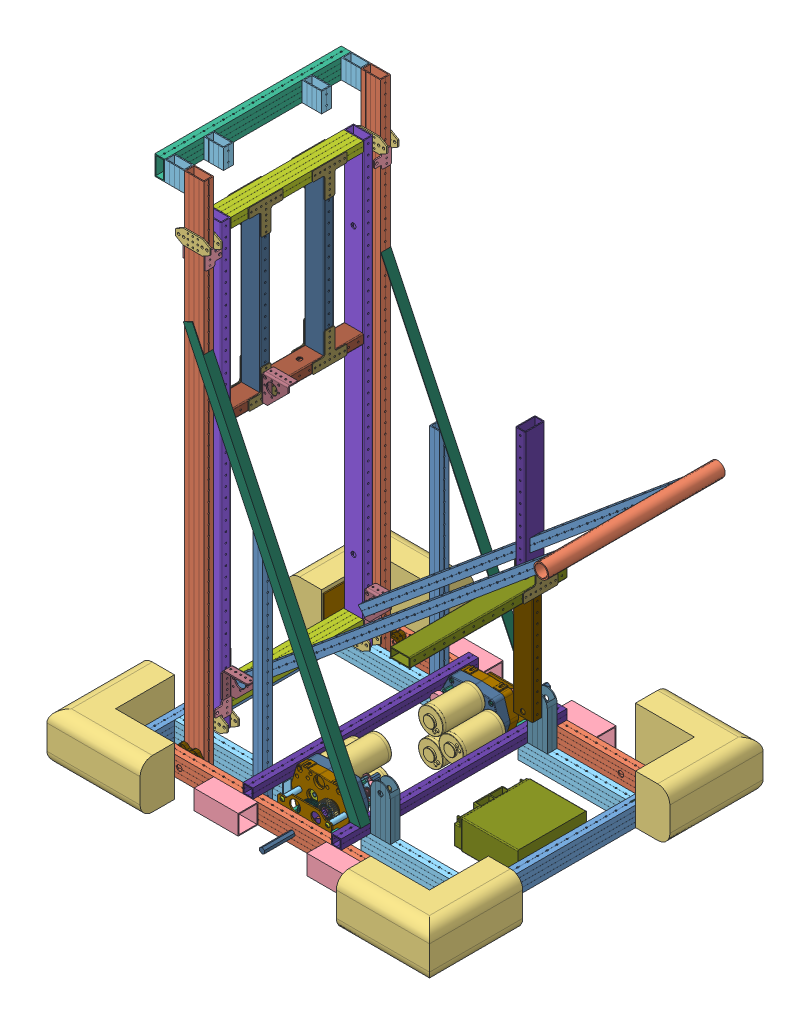
SolidWorks assembly Test Robot 4, configuration Default. Lengths in mm.
Overall size (1132.98 1353.06 863.6).
309 component instances, 94 part files, 31 mates.
Components (placement in the parent):
- Test Base 4-1: Test Base 4 [Default] at (-277.5499 -97.123 227.8911) size (990.6 641.86 863.6)
  - Base Rear Rail-1: Base Rear Rail [Default] at (282.1219 360.9185 104.1623) size (25.4 50.8 685.8)
  - Base Side Rail-1: Base Side Rail [Default] at (1044.1219 360.9185 789.9623) x (0 0 1) z (-1 0 0) size (25.4 50.8 762)
  - Base Side Rail-2: Base Side Rail [Default] at (1044.1219 360.9185 231.1623) x (0 0 1) z (-1 0 0) size (25.4 50.8 762)
  - Blue Bumper-1: Blue Bumper [Default] at (1171.1219 335.5185 942.3623) x (0 0 -1) z (1 0 0) size (241.3 127 241.3)
  - Blue Bumper-2: Blue Bumper [Default] at (1171.1219 335.5185 78.7623) x (-1 0 0) z (0 0 -1) size (241.3 127 241.3)
  - Bumper Support Bar-2: Bumper Support Bar [Default] at (879.0219 335.5185 166.0294) x (0 0 1) z (-1 0 0) size (50.8 50.8 114.3)
  - Bumper Support Bar-4: Bumper Support Bar [Default] at (586.9219 335.5185 166.0294) x (0 0 1) z (-1 0 0) size (50.8 50.8 114.3)
  - Bumper Support Bar-7: Bumper Support Bar [Default] at (586.9219 335.5185 801.0294) x (0 0 1) z (-1 0 0) size (50.8 50.8 114.3)
  - Bumper Support Bar-8: Bumper Support Bar [Default] at (879.0219 335.5185 801.0294) x (0 0 1) z (-1 0 0) size (50.8 50.8 114.3)
  - Base Side Rail Internal-1: Base Side Rail Internal [Default] at (-175.0781 360.9185 713.7623) x (0 0 -1) z (1 0 0) size (25.4 50.8 279.4)
  - Base Side Rail Internal-4: Base Side Rail Internal [Default] at (1044.1219 360.9185 307.3623) x (0 0 1) z (-1 0 0) size (25.4 50.8 279.4)
  - Base Front Rail-1: Base Front Rail [Default] at (1069.5219 360.9185 104.1623) size (25.4 50.8 152.4)
  - 3 CIM Ball Shifter with WCD Output-1: 3 CIM Ball Shifter with WCD Output [Default] at (711.3612 400.7203 682.3171) x (0 1 0) z (0 0 1) size (169.11 183.68 312.65)
    - 217-2733-001 Rev2-1: 217-2733-001 Rev2 [Default] at (0 53.4162 37.6682) x (0 0 1) z (-0.00054 -1 0) size (7.11 24.61 24.61)
    - 217-2733-001 Rev2-2: 217-2733-001 Rev2 [Default] at (0 53.4162 7.9248) x (0 0 -1) z (-0.038475 0.99926 0) size (7.11 24.61 24.61)
    - 217-2731-001 Rev2-1: 217-2731-001 Rev2 [Default] at (0 0 0.0381) x (-0.099212 0.995066 0) z (0.995066 0.099212 0) size (31.12 7.94 31.12)
    - 217-2789-001 Rev2-1: 217-2789-001 Rev2 [Default] at (0 0 43.2943) x (0 0 -1) z (-0.58471 0.811243 0) size (11.1 38.4 38.4)
    - 217-2778-001 Rev2_NCQ8A075-050M_1-1: 217-2778-001 Rev2_NCQ8A075-050M_1 [Default] at (0 0 -53.848) x (-0.707107 0.707107 0) z (0 0 1) size (31.75 33.34 39.88)
      - 217-2778-002_075A-1: 217-2778-002_075A [Default] at origin size (31.75 33.34 26.92)
      - 217-2778-003_075M-1: 217-2778-003_075M [Default] at (0 0 -8.85) x (0.866025 -0.5 0) z (0 0 1) size (18.95 18.95 35.27)
      - 217-2778-004_075-1: 217-2778-004_075 [Default] at (0 0 10.362) size (21 20.74 0.97)
    - 217-2428-012 Rev2-1: 217-2428-012 Rev2 [Default] at (0 0 -40.386) size (63.5 22.23 2.29)
    - 217-2428-005 Rev1-1: 217-2428-005 Rev1 [Default] at (25.4 0 -19.05) x (-0.557362 -0.83027 0) z (-0.83027 0.557362 0) size (7.33 38.98 6.35)
    - 217-2428-005 Rev1-2: 217-2428-005 Rev1 [Default] at (-25.4 0 -19.05) x (0.667436 0.744667 0) z (0.744667 -0.667436 0) size (7.33 38.98 6.35)
    - SCREW-832-0375-1: SCREW-832-0375 [Default] at (25.4 0 -42.5958) x (0 0 1) z (-0.875404 0.483392 0) size (11.73 7.92 7.92)
    - SCREW-832-0375-2: SCREW-832-0375 [Default] at (-25.4 0 -42.5958) x (0 0 1) z (-0.966319 0.257347 0) size (11.73 7.92 7.92)
    - SCREW-832-0375-3: SCREW-832-0375 [Default] at (25.4 0 5.3848) x (0 0 -1) z (1 0 0) size (11.73 7.92 7.92)
    - SCREW-832-0375-4: SCREW-832-0375 [Default] at (-25.4 0 5.3848) x (0 0 -1) z (0.941463 -0.337115 0) size (11.73 7.92 7.92)
    - SBS1_SBS-0632-0250-1: SBS1_SBS-0632-0250 [Default] at (15.494 0 -36.2458) x (0 0 -1) z (0.854303 -0.519775 0) size (8.57 6.68 6.65)
    - SBS1_SBS-0632-0250-2: SBS1_SBS-0632-0250 [Default] at (-15.494 0 -36.2458) x (0 0 -1) z (0.854303 -0.519775 0) size (8.57 6.68 6.65)
    - 217-4098-100 Rev1-1: 217-4098-100 Rev1 [Default] at (0 0 -16.927) x (-0.503316 0.864103 0) z (0 0 1) size (18.03 19.79 22.46)
      - 217-4098-006 Rev2-1: 217-4098-006 Rev2 [Default] at (0 0 -4.6312) x (0 -1 0) z (0 0 -1) size (18.09 11.02 22.46)
      - 217-4098-006 Rev2-2: 217-4098-006 Rev2 [Default] at (0 0 -4.6312) x (0 1 0) z (0 0 -1) size (18.09 11.02 22.46)
      - 217-3489-001 Rev1-1: 217-3489-001 Rev1 [Default] at (0 0 -4.6312) x (0 0 1) z (-0.980217 -0.197926 0) size (4.77 12.7 12.7)
      - 97633A130_97633A130_grv-1: 97633A130_97633A130_grv [Default] at (0 0 -7.33) x (0 0 -1) z (0.979861 0.199683 0) size (0.64 8.74 7.34)
      - 91251A107_91251A107-1: 91251A107_91251A107 [Default] at (-4.8375 -6.735 -9.4343) x (0 0.863883 -0.503692) z (-1 0 0) size (4.65 4.65 10.79)
      - 91251A107_91251A107-2: 91251A107_91251A107 [Default] at (4.8375 6.735 -9.4343) x (0 0.470889 -0.882193) z (1 0 0) size (4.65 4.65 10.79)
    - 217-2428-017 Rev2-1: 217-2428-017 Rev2 [Default] at (12.7 -21.997 -3.614) x (-0.578458 -0.815712 0) z (0 0 -1) size (14.73 14.73 7.37)
    - 217-2428-016 Rev3_Spur01-1: 217-2428-016 Rev3_Spur01 [Default] at (0 0 -3.614) x (0.873157 -0.48744 0) z (0 0 1) size (40.67 40.74 13.32)
    - 217-2428-019 Rev1-1: 217-2428-019 Rev1 [Default] at (12.7 -21.997 -20.6248) x (0.866025 0.5 0) z (0 0 1) size (50.8 19.05 1.57)
    - 217-2428-006 Rev1-1: 217-2428-006 Rev1 [Default] at (32.079 -14.2875 -9.525) x (-0.752416 0.658689 0) z (0.658689 0.752416 0) size (7.33 19.93 6.35)
    - 217-2428-006 Rev1-2: 217-2428-006 Rev1 [Default] at (-3.6662 -34.925 -9.525) x (0.84498 0.534798 0) z (0.534798 -0.84498 0) size (7.33 19.93 6.35)
    - SCREW-832-0375-5: SCREW-832-0375 [Default] at (32.079 -14.2875 4.7498) x (0 0 -1) z (0.980613 0.195955 0) size (11.73 7.92 7.92)
    - SCREW-832-0375-6: SCREW-832-0375 [Default] at (-3.6662 -34.925 5.3848) x (0 0 -1) z (-0.672515 -0.740083 0) size (11.73 7.92 7.92)
    - SCREW-832-0375-7: SCREW-832-0375 [Default] at (-3.6662 -34.925 -22.8346) x (0 0 1) z (0.948865 0.315681 0) size (11.73 7.92 7.92)
    - SCREW-832-0375-8: SCREW-832-0375 [Default] at (32.079 -14.2875 -22.8346) x (0 0 1) z (-0.875404 0.483392 0) size (11.73 7.92 7.92)
    - 217-2614-001_12t-1: 217-2614-001_12t [Default] at (36.9798 39.6868 15.8623) x (-0.087156 0.996195 0) z (0 0 1) size (18.29 18.29 19)
    - 217-2761-001 rev1-1: 217-2761-001 rev1 [Default] at (33.1943 39.3556 16.1) x (0.087156 -0.996195 0) z (0 0 1) size (2 2 20)
    - 217-2761-001 rev1-2: 217-2761-001 rev1 [Default] at (-40.7653 40.018 16.1) x (0.087156 0.996195 0) z (0 0 1) size (2 2 20)
    - 217-2614-001_12t-2: 217-2614-001_12t [Default] at (-36.9798 39.6868 15.8623) x (0.087156 0.996195 0) z (0 0 1) size (18.29 18.29 19)
    - 217-2614-001_12t-3: 217-2614-001_12t [Default] at (0 92.8624 15.8623) x (0.97459 0.223996 0) z (0 0 1) size (18.29 18.29 19)
    - 217-2761-001 rev1-3: 217-2761-001 rev1 [Default] at (-0.8512 96.5658 16.1) x (0.97459 0.223996 0) z (0 0 1) size (2 2 20)
    - 217-3195-002 rev2-1: 217-3195-002 rev2 [Default] at (0 0 50.546) x (-1 0 0) z (0 0 -1) size (114.31 152.24 24.96)
    - 217-3195-001 Rev1-1: 217-3195-001 Rev1 [Default] at origin size (113.41 152.24 26.86)
    - Nylock Nut_NNY2520-ZC-1: Nylock Nut_NNY2520-ZC [Default] at (48.8823 73.025 37.846) x (0 0.866025 -0.5) z (-1 0 0) size (12.85 11.89 7.62)
    - Nylock Nut_NNY2520-ZC-2: Nylock Nut_NNY2520-ZC [Default] at (48.8823 -3.175 37.846) x (0 0 -1) z (-1 0 0) size (12.85 11.89 7.62)
    - Nylock Nut_NNY2520-ZC-3: Nylock Nut_NNY2520-ZC [Default] at (44.45 85.725 7.8613) x (0 1 0) z (0 0 -1) size (12.85 11.89 7.62)
    - 276-1027-001-1: 276-1027-001 [Default] at (47.625 58.1787 6.35) x (0 1 0) z (-1 0 0) size (8.61 5.64 9.94)
    - 276-1027-001-2: 276-1027-001 [Default] at (-47.625 58.1787 6.35) x (0 -1 0) z (1 0 0) size (8.61 5.64 9.94)
    - SCREW-832-1750-1: SCREW-832-1750 [Default] at (-47.625 58.1787 47.0408) x (0 0 -1) z (-0.960822 -0.277167 0) size (46.66 7.92 7.92)
    - SCREW-832-1750-2: SCREW-832-1750 [Default] at (47.625 58.1787 47.0408) x (0 0 -1) z (-0.960822 -0.277167 0) size (46.66 7.92 7.92)
    - Nylock Nut_NNY2520-ZC-4: Nylock Nut_NNY2520-ZC [Default] at (44.45 -15.875 7.8613) x (0 1 0) z (0 0 -1) size (12.85 11.89 7.62)
    - 217-2428-004 Rev3-1: 217-2428-004 Rev3 [Default] at (0 53.4162 22.7711) x (-0.709585 0.70462 0) z (0 0 1) size (11 9.53 43.92)
    - SBS1_SBS-2520-1625SS-1: SBS1_SBS-2520-1625SS [Default] at (44.45 85.725 42.4688) x (0 0 -1) z (-0.251219 0.96793 0) size (45.3 11.2 11.18)
    - SBS1_SBS-2520-1625SS-2: SBS1_SBS-2520-1625SS [Default] at (44.45 -15.875 42.4688) x (0 0 -1) z (-0.251219 0.96793 0) size (45.3 11.2 11.18)
    - SBS1_SBS2520-1750-1: SBS1_SBS2520-1750 [Default] at (-44.45 85.725 7.4422) x (0 0 1) z (-0.031478 0.999504 0) size (48.48 11.22 11.17)
    - SBS1_SBS2520-1750-2: SBS1_SBS2520-1750 [Default] at (-44.45 -15.875 7.4422) x (0 0 1) z (-0.937114 -0.349025 0) size (48.48 11.22 11.17)
    - 217-2428-021 Rev1-1: 217-2428-021 Rev1 [Default] at (0 53.4162 9.5123) x (0.451333 -0.892356 0) z (0 0 1) size (15.88 15.88 3.17)
    - 217-2428-029 Rev1-1: 217-2428-029 Rev1 [Default] at (0 53.4162 36.957) x (0.999846 0.017557 0) z (0 0 1) size (15.88 15.88 1.12)
    - Grayhill Lock Washer-1: Grayhill Lock Washer [Default] at (12.7 -21.997 -18.6817) x (0.467173 -0.884166 0) z (0 0 1) size (19.69 19.69 0.74)
    - Grayhill Nut-1: Grayhill Nut [Default] at (12.7 -21.997 -17.0434) x (0.984088 0.177684 0) z (0 0 1) size (18.33 15.88 2.54)
    - 217-2000-1: 217-2000 [Default] at (0 92.8624 0) x (0 0 -1) z (0.223996 -0.97459 0) size (150.2 64.01 64.01)
    - 217-2000-2: 217-2000 [Default] at (-36.9798 39.6868 0) x (0 0 -1) z (0.996195 -0.087156 0) size (150.2 64.01 64.01)
    - 217-2000-3: 217-2000 [Default] at (36.9798 39.6868 0) x (0 0 -1) z (0.996195 0.087156 0) size (150.2 64.01 64.01)
    - Grahill Encoder-1: Grahill Encoder [Default] at (12.7 -21.997 -16.1798) x (-0.580071 0.814566 0) z (-0.814566 -0.580071 0) size (31.75 31.12 31.75)
    - 217-3195-009 Rev1_wcd 2-1: 217-3195-009 Rev1_wcd 2 [Default] at (0 85.725 50.546) x (-0.998427 -0.056065 0) z (0 0 1) size (12.7 12.7 41.27)
    - 217-3195-006 Rev1_WCD-1: 217-3195-006 Rev1_WCD [Default] at (-44.45 85.725 44.1452) x (0.5 0.866025 0) z (0 0 1) size (12.7 14.66 47.62)
    - 217-3195-009 Rev1_wcd 2-2: 217-3195-009 Rev1_wcd 2 [Default] at (0 -31.75 50.546) x (0.947633 0.319361 0) z (0 0 1) size (12.7 12.7 41.27)
    - 217-3195-006 Rev1_WCD-2: 217-3195-006 Rev1_WCD [Default] at (-44.45 -15.875 44.1452) x (0.5 -0.866025 0) z (0 0 1) size (12.7 14.66 47.62)
    - Nylock Nut_NNY2520-ZC-5: Nylock Nut_NNY2520-ZC [Default] at (0 -31.75 45.0723) x (-0.5 0.866025 0) z (0 0 -1) size (12.85 11.89 7.62)
    - Nylock Nut_NNY2520-ZC-6: Nylock Nut_NNY2520-ZC [Default] at (0 85.725 45.0723) x (-0.5 0.866025 0) z (0 0 -1) size (12.85 11.89 7.62)
    - SBS1_SBS-2520-2250-1: SBS1_SBS-2520-2250 [Default] at (0 -31.75 98.298) x (0 0 -1) z (-0.933488 -0.358607 0) size (61.18 11.22 11.17)
    - SBS1_SBS2520-0625ZC-1: SBS1_SBS2520-0625ZC [Default] at (-44.45 85.725 98.298) x (0 0 -1) z (0.400817 0.916158 0) size (19.57 11.22 11.17)
    - SBS1_SBS2520-0625ZC-2: SBS1_SBS2520-0625ZC [Default] at (-44.45 -15.875 98.298) x (0 0 -1) z (-0.75178 -0.659414 0) size (19.57 11.22 11.17)
    - SBS1_SBS-2520-2250-2: SBS1_SBS-2520-2250 [Default] at (0 85.725 98.298) x (0 0 -1) z (0.056677 -0.998393 0) size (61.18 11.22 11.17)
    - 217-3195-003 rev2-1: 217-3195-003 rev2 [Default] at (0 0 94.9452) size (88.62 139.7 3.17)
    - 217-2617-003 Rev1-1: 217-2617-003 Rev1 [Default] at (-39.878 35.5392 121.8535) x (-0.5 -0.866025 0) z (0 0 1) size (14.66 12.7 152.4)
    - 217-3109-001 Rev1-1: 217-3109-001 Rev1 [Default] at (-39.878 35.5392 49.1808) x (0 0 1) z (0.312889 -0.94979 0) size (7.94 28.57 28.57)
    - 217-2734-001 Rev3-1: 217-2734-001 Rev3 [Default] at (-39.878 35.5392 98.1202) x (1 0 0) z (0 1 0) size (31.12 7.94 31.12)
    - 217-2617-004 Rev1_97431A340_grv-1: 217-2617-004 Rev1_97431A340_grv [Default] at (-39.878 35.5392 54.8961) x (0 0 1) z (-0.124043 -0.992277 0) size (1.07 20.42 18.58)
    - 217-2617-004 Rev1_97431A340_grv-2: 217-2617-004 Rev1_97431A340_grv [Default] at (0 0 69.215) x (0 0 1) z (-0.124043 -0.992277 0) size (1.07 20.42 18.58)
    - 217-2702-001_20t-1: 217-2702-001_20t [Default] at (0 0 62.357) x (0.998435 0.055929 0) z (0 0 1) size (28.2 28.2 12.65)
    - 217-2715-002 Rev1_64t-1: 217-2715-002 Rev1_64t [Default] at (-39.878 35.5392 61.7541) x (0.866025 -0.5 0) z (0 0 1) size (84.3 84.3 12.65)
    - 217-2704-001_24-1: 217-2704-001_24 [Default] at (0 0 62.357) x (0.450781 0.892635 0) z (0 0 -1) size (33.29 33.29 12.65)
    - 217-2714-002 Rev1_60t-1: 217-2714-002 Rev1_60t [Default] at (-39.878 35.5392 61.7541) x (0.866025 -0.5 0) z (0 0 1) size (78.95 78.95 12.65)
    - 217-3221-002 Rev1-1: 217-3221-002 Rev1 [Default] at (-39.878 35.5392 61.7414) x (0 -1 0) z (0 0 1) size (71.39 71.45 12.62)
    - 217-2705-001_30t-1: 217-2705-001_30t [Default] at (0 0 62.357) x (0.547654 -0.836705 0) z (0 0 1) size (41.01 41.12 12.65)
    - 217-2712-002 Rev1_50t-1: 217-2712-002 Rev1_50t [Default] at (-39.878 35.5392 61.7541) x (0.866025 -0.5 0) z (0 0 1) size (66.7 66.76 12.65)
    - 217-2706-001_34t-1: 217-2706-001_34t [Default] at (0 0 62.357) x (0.998435 0.055929 0) z (0 0 1) size (46.46 46.56 12.65)
    - 217-3288-001 Rev3-1: 217-3288-001 Rev3 [Default] at (0 0 0.0889) x (0.055929 -0.998435 0) z (0 0 1) size (99.51 99.53 98.3)
      - 217-2428-008 Rev2-1: 217-2428-008 Rev2 [Default] at (0 0 10.2679) size (31.75 31.75 1.59)
      - 217-2428-028 Rev1_97633A250-1: 217-2428-028 Rev1_97633A250 [Default] at (0 0 37.1221) x (0 0 1) z (0.9357 -0.352797 0) size (1.07 23.39 21.18)
      - 217-4099-000 Rev2_high gear-1: 217-4099-000 Rev2_high gear [Default] x (-1 0 0) z (0 0 1) size (22.23 22.23 98.3)
        - 217-4098-005 Rev1_91612A226-1: 217-4098-005 Rev1_91612A226 [Default] at (0 0 46.2661) x (-0.144757 0 0.989467) z (0 -1 0) size (3.02 3.15 18.22)
        - 217-4098-003 Rev2-1: 217-4098-003 Rev2 [Default] x (1 0 0) z (0 0 -1) size (22.23 22.23 55.94)
        - 217-4099-002 Rev3-1: 217-4099-002 Rev3 [Default] at (0 0 53.467) x (0 0 1) z (-1 0 0) size (40.96 12.73 14.67)
        - 217-4098-004 Rev1-1: 217-4098-004 Rev1 [Default] at (0 0 14.2494) x (0.393904 0.919152 0) z (0 0 1) size (11.68 11.68 56)
      - 217-2428-007 Rev1-1: 217-2428-007 Rev1 [Default] at (7.809 4.5085 14.2494) x (-0.69071 0.455693 -0.561483) z (-0.67559 -0.683536 0.276329) size (6.35 6.35 6.35)
      - 217-2428-007 Rev1-2: 217-2428-007 Rev1 [Default] at (5.4343 3.1375 26.9494) x (-0.162331 -0.978398 0.128005) z (0.857281 -0.204076 -0.472676) size (6.35 6.35 6.35)
      - 217-3212-101 Rev1-1: 217-3212-101 Rev1 [Default] at (-11.5751 10.4131 45.3224) x (0.923728 0.383049 0) z (0 0 -1) size (46.46 46.56 12.7)
        - 217-2428-022 Rev1-1: 217-2428-022 Rev1 [Default] at (6.7035 14.0527 24.6087) size (28.57 28.57 6.1)
        - 217-3212-001 Rev1_34t-1: 217-3212-001 Rev1_34t [Default] at (6.7035 14.0527 27.9107) size (46.46 46.56 11.11)
      - 217-3222-101 Rev1-1: 217-3222-101 Rev1 [Default] at (21.0941 -5.2804 52.7371) x (-0.889163 -0.457591 0) z (0 0 -1) size (73.87 73.92 12.7)
        - 217-2428-022 Rev1-1: 217-2428-022 Rev1 [Default] at (16.3398 14.3476 19.3234) size (28.57 28.57 6.1)
        - 217-3222-001 Rev1_Spur01-1: 217-3222-001 Rev1_Spur01 [Default] at (16.3398 14.3476 22.6254) x (0.999377 0.0353 0) z (0 0 1) size (71.39 71.45 11.11)
      - 217-2428-007 Rev1-3: 217-2428-007 Rev1 [Default] at (-5.4343 3.1375 26.9494) x (0.928483 0.348617 0.128005) z (-0.251905 0.844465 -0.472676) size (6.35 6.35 6.35)
      - 217-2428-007 Rev1-4: 217-2428-007 Rev1 [Default] at (0 -6.275 26.9494) x (-0.766153 0.629782 0.128005) z (-0.605376 -0.640389 -0.472676) size (6.35 6.35 6.35)
      - 217-2428-007 Rev1-5: 217-2428-007 Rev1 [Default] at (-7.809 4.5085 14.2494) x (-0.049287 -0.826019 -0.561483) z (0.929754 -0.24331 0.276329) size (6.35 6.35 6.35)
      - 217-2428-007 Rev1-6: 217-2428-007 Rev1 [Default] at (0 -9.017 14.2494) x (0.739997 0.370326 -0.561483) z (-0.254164 0.926846 0.276329) size (6.35 6.35 6.35)
    - 217-3210-001 Rev1_30t-1: 217-3210-001 Rev1_30t [Default] at (0 53.4162 30.0736) x (-0.966828 0.255427 0) z (0 0 1) size (41.01 41.12 12.65)
    - 217-2711-002 Rev1_50t-1: 217-2711-002 Rev1_50t [Default] at (0 53.4162 17.4244) x (0.262208 -0.965011 0) z (0 0 1) size (66.7 66.76 12.65)
  - 3 CIM Ball Shifter with WCD Output-2: 3 CIM Ball Shifter with WCD Output [Default] at (640.2827 400.7203 338.8075) x (0 1 0) z (0 0 -1) size (169.11 183.68 312.65)
    - 217-2733-001 Rev2-1: 217-2733-001 Rev2 [Default] at (0 53.4162 37.6682) x (0 0 1) z (-0.00054 -1 0) size (7.11 24.61 24.61)
    - 217-2733-001 Rev2-2: 217-2733-001 Rev2 [Default] at (0 53.4162 7.9248) x (0 0 -1) z (-0.038475 0.99926 0) size (7.11 24.61 24.61)
    - 217-2731-001 Rev2-1: 217-2731-001 Rev2 [Default] at (0 0 0.0381) x (-0.099212 0.995066 0) z (0.995066 0.099212 0) size (31.12 7.94 31.12)
    - 217-2789-001 Rev2-1: 217-2789-001 Rev2 [Default] at (0 0 43.2943) x (0 0 -1) z (-0.58471 0.811243 0) size (11.1 38.4 38.4)
    - 217-2778-001 Rev2_NCQ8A075-050M_1-1: 217-2778-001 Rev2_NCQ8A075-050M_1 [Default] at (0 0 -53.848) x (-0.707107 0.707107 0) z (0 0 1) size (31.75 33.34 39.88)
      - 217-2778-002_075A-1: 217-2778-002_075A [Default] at origin size (31.75 33.34 26.92)
      - 217-2778-003_075M-1: 217-2778-003_075M [Default] at (0 0 -8.85) x (0.866025 -0.5 0) z (0 0 1) size (18.95 18.95 35.27)
      - 217-2778-004_075-1: 217-2778-004_075 [Default] at (0 0 10.362) size (21 20.74 0.97)
    - 217-2428-012 Rev2-1: 217-2428-012 Rev2 [Default] at (0 0 -40.386) size (63.5 22.23 2.29)
    - 217-2428-005 Rev1-1: 217-2428-005 Rev1 [Default] at (25.4 0 -19.05) x (-0.557362 -0.83027 0) z (-0.83027 0.557362 0) size (7.33 38.98 6.35)
    - 217-2428-005 Rev1-2: 217-2428-005 Rev1 [Default] at (-25.4 0 -19.05) x (0.667436 0.744667 0) z (0.744667 -0.667436 0) size (7.33 38.98 6.35)
    - SCREW-832-0375-1: SCREW-832-0375 [Default] at (25.4 0 -42.5958) x (0 0 1) z (-0.875404 0.483392 0) size (11.73 7.92 7.92)
    - SCREW-832-0375-2: SCREW-832-0375 [Default] at (-25.4 0 -42.5958) x (0 0 1) z (-0.966319 0.257347 0) size (11.73 7.92 7.92)
    - SCREW-832-0375-3: SCREW-832-0375 [Default] at (25.4 0 5.3848) x (0 0 -1) z (1 0 0) size (11.73 7.92 7.92)
    - SCREW-832-0375-4: SCREW-832-0375 [Default] at (-25.4 0 5.3848) x (0 0 -1) z (0.941463 -0.337115 0) size (11.73 7.92 7.92)
    - SBS1_SBS-0632-0250-1: SBS1_SBS-0632-0250 [Default] at (15.494 0 -36.2458) x (0 0 -1) z (0.854303 -0.519775 0) size (8.57 6.68 6.65)
    - SBS1_SBS-0632-0250-2: SBS1_SBS-0632-0250 [Default] at (-15.494 0 -36.2458) x (0 0 -1) z (0.854303 -0.519775 0) size (8.57 6.68 6.65)
    - 217-4098-100 Rev1-1: 217-4098-100 Rev1 [Default] at (0 0 -16.927) x (-0.503316 0.864103 0) z (0 0 1) size (18.03 19.79 22.46)
      - 217-4098-006 Rev2-1: 217-4098-006 Rev2 [Default] at (0 0 -4.6312) x (0 -1 0) z (0 0 -1) size (18.09 11.02 22.46)
      - 217-4098-006 Rev2-2: 217-4098-006 Rev2 [Default] at (0 0 -4.6312) x (0 1 0) z (0 0 -1) size (18.09 11.02 22.46)
      - 217-3489-001 Rev1-1: 217-3489-001 Rev1 [Default] at (0 0 -4.6312) x (0 0 1) z (-0.980217 -0.197926 0) size (4.77 12.7 12.7)
      - 97633A130_97633A130_grv-1: 97633A130_97633A130_grv [Default] at (0 0 -7.33) x (0 0 -1) z (0.979861 0.199683 0) size (0.64 8.74 7.34)
      - 91251A107_91251A107-1: 91251A107_91251A107 [Default] at (-4.8375 -6.735 -9.4343) x (0 0.863883 -0.503692) z (-1 0 0) size (4.65 4.65 10.79)
      - 91251A107_91251A107-2: 91251A107_91251A107 [Default] at (4.8375 6.735 -9.4343) x (0 0.470889 -0.882193) z (1 0 0) size (4.65 4.65 10.79)
    - 217-2428-017 Rev2-1: 217-2428-017 Rev2 [Default] at (12.7 -21.997 -3.614) x (-0.578458 -0.815712 0) z (0 0 -1) size (14.73 14.73 7.37)
    - 217-2428-016 Rev3_Spur01-1: 217-2428-016 Rev3_Spur01 [Default] at (0 0 -3.614) x (0.873157 -0.48744 0) z (0 0 1) size (40.67 40.74 13.32)
    - 217-2428-019 Rev1-1: 217-2428-019 Rev1 [Default] at (12.7 -21.997 -20.6248) x (0.866025 0.5 0) z (0 0 1) size (50.8 19.05 1.57)
    - 217-2428-006 Rev1-1: 217-2428-006 Rev1 [Default] at (32.079 -14.2875 -9.525) x (-0.752416 0.658689 0) z (0.658689 0.752416 0) size (7.33 19.93 6.35)
    - 217-2428-006 Rev1-2: 217-2428-006 Rev1 [Default] at (-3.6662 -34.925 -9.525) x (0.84498 0.534798 0) z (0.534798 -0.84498 0) size (7.33 19.93 6.35)
    - SCREW-832-0375-5: SCREW-832-0375 [Default] at (32.079 -14.2875 4.7498) x (0 0 -1) z (0.980613 0.195955 0) size (11.73 7.92 7.92)
    - SCREW-832-0375-6: SCREW-832-0375 [Default] at (-3.6662 -34.925 5.3848) x (0 0 -1) z (-0.672515 -0.740083 0) size (11.73 7.92 7.92)
    - SCREW-832-0375-7: SCREW-832-0375 [Default] at (-3.6662 -34.925 -22.8346) x (0 0 1) z (0.948865 0.315681 0) size (11.73 7.92 7.92)
    - SCREW-832-0375-8: SCREW-832-0375 [Default] at (32.079 -14.2875 -22.8346) x (0 0 1) z (-0.875404 0.483392 0) size (11.73 7.92 7.92)
    - 217-2614-001_12t-1: 217-2614-001_12t [Default] at (36.9798 39.6868 15.8623) x (-0.087156 0.996195 0) z (0 0 1) size (18.29 18.29 19)
    - 217-2761-001 rev1-1: 217-2761-001 rev1 [Default] at (33.1943 39.3556 16.1) x (0.087156 -0.996195 0) z (0 0 1) size (2 2 20)
    - 217-2761-001 rev1-2: 217-2761-001 rev1 [Default] at (-40.7653 40.018 16.1) x (0.087156 0.996195 0) z (0 0 1) size (2 2 20)
    - 217-2614-001_12t-2: 217-2614-001_12t [Default] at (-36.9798 39.6868 15.8623) x (0.087156 0.996195 0) z (0 0 1) size (18.29 18.29 19)
    - 217-2614-001_12t-3: 217-2614-001_12t [Default] at (0 92.8624 15.8623) x (0.97459 0.223996 0) z (0 0 1) size (18.29 18.29 19)
    - 217-2761-001 rev1-3: 217-2761-001 rev1 [Default] at (-0.8512 96.5658 16.1) x (0.97459 0.223996 0) z (0 0 1) size (2 2 20)
    - 217-3195-002 rev2-1: 217-3195-002 rev2 [Default] at (0 0 50.546) x (-1 0 0) z (0 0 -1) size (114.31 152.24 24.96)
    - 217-3195-001 Rev1-1: 217-3195-001 Rev1 [Default] at origin size (113.41 152.24 26.86)
    - Nylock Nut_NNY2520-ZC-1: Nylock Nut_NNY2520-ZC [Default] at (48.8823 73.025 37.846) x (0 0.866025 -0.5) z (-1 0 0) size (12.85 11.89 7.62)
    - Nylock Nut_NNY2520-ZC-2: Nylock Nut_NNY2520-ZC [Default] at (48.8823 -3.175 37.846) x (0 0 -1) z (-1 0 0) size (12.85 11.89 7.62)
    - Nylock Nut_NNY2520-ZC-3: Nylock Nut_NNY2520-ZC [Default] at (44.45 85.725 7.8613) x (0 1 0) z (0 0 -1) size (12.85 11.89 7.62)
    - 276-1027-001-1: 276-1027-001 [Default] at (47.625 58.1787 6.35) x (0 1 0) z (-1 0 0) size (8.61 5.64 9.94)
    - 276-1027-001-2: 276-1027-001 [Default] at (-47.625 58.1787 6.35) x (0 -1 0) z (1 0 0) size (8.61 5.64 9.94)
    - SCREW-832-1750-1: SCREW-832-1750 [Default] at (-47.625 58.1787 47.0408) x (0 0 -1) z (-0.960822 -0.277167 0) size (46.66 7.92 7.92)
    - SCREW-832-1750-2: SCREW-832-1750 [Default] at (47.625 58.1787 47.0408) x (0 0 -1) z (-0.960822 -0.277167 0) size (46.66 7.92 7.92)
    - Nylock Nut_NNY2520-ZC-4: Nylock Nut_NNY2520-ZC [Default] at (44.45 -15.875 7.8613) x (0 1 0) z (0 0 -1) size (12.85 11.89 7.62)
    - 217-2428-004 Rev3-1: 217-2428-004 Rev3 [Default] at (0 53.4162 22.7711) x (-0.709585 0.70462 0) z (0 0 1) size (11 9.53 43.92)
    - SBS1_SBS-2520-1625SS-1: SBS1_SBS-2520-1625SS [Default] at (44.45 85.725 42.4688) x (0 0 -1) z (-0.251219 0.96793 0) size (45.3 11.2 11.18)
    - SBS1_SBS-2520-1625SS-2: SBS1_SBS-2520-1625SS [Default] at (44.45 -15.875 42.4688) x (0 0 -1) z (-0.251219 0.96793 0) size (45.3 11.2 11.18)
    - SBS1_SBS2520-1750-1: SBS1_SBS2520-1750 [Default] at (-44.45 85.725 7.4422) x (0 0 1) z (-0.031478 0.999504 0) size (48.48 11.22 11.17)
    - SBS1_SBS2520-1750-2: SBS1_SBS2520-1750 [Default] at (-44.45 -15.875 7.4422) x (0 0 1) z (-0.937114 -0.349025 0) size (48.48 11.22 11.17)
    - 217-2428-021 Rev1-1: 217-2428-021 Rev1 [Default] at (0 53.4162 9.5123) x (0.451333 -0.892356 0) z (0 0 1) size (15.88 15.88 3.17)
    - 217-2428-029 Rev1-1: 217-2428-029 Rev1 [Default] at (0 53.4162 36.957) x (0.999846 0.017557 0) z (0 0 1) size (15.88 15.88 1.12)
    - Grayhill Lock Washer-1: Grayhill Lock Washer [Default] at (12.7 -21.997 -18.6817) x (0.467173 -0.884166 0) z (0 0 1) size (19.69 19.69 0.74)
    - Grayhill Nut-1: Grayhill Nut [Default] at (12.7 -21.997 -17.0434) x (0.984088 0.177684 0) z (0 0 1) size (18.33 15.88 2.54)
    - 217-2000-1: 217-2000 [Default] at (0 92.8624 0) x (0 0 -1) z (0.223996 -0.97459 0) size (150.2 64.01 64.01)
    - 217-2000-2: 217-2000 [Default] at (-36.9798 39.6868 0) x (0 0 -1) z (0.996195 -0.087156 0) size (150.2 64.01 64.01)
    - 217-2000-3: 217-2000 [Default] at (36.9798 39.6868 0) x (0 0 -1) z (0.996195 0.087156 0) size (150.2 64.01 64.01)
    - Grahill Encoder-1: Grahill Encoder [Default] at (12.7 -21.997 -16.1798) x (-0.580071 0.814566 0) z (-0.814566 -0.580071 0) size (31.75 31.12 31.75)
    - 217-3195-009 Rev1_wcd 2-1: 217-3195-009 Rev1_wcd 2 [Default] at (0 85.725 50.546) x (-0.998427 -0.056065 0) z (0 0 1) size (12.7 12.7 41.27)
    - 217-3195-006 Rev1_WCD-1: 217-3195-006 Rev1_WCD [Default] at (-44.45 85.725 44.1452) x (0.5 0.866025 0) z (0 0 1) size (12.7 14.66 47.62)
    - 217-3195-009 Rev1_wcd 2-2: 217-3195-009 Rev1_wcd 2 [Default] at (0 -31.75 50.546) x (0.947633 0.319361 0) z (0 0 1) size (12.7 12.7 41.27)
    - 217-3195-006 Rev1_WCD-2: 217-3195-006 Rev1_WCD [Default] at (-44.45 -15.875 44.1452) x (0.5 -0.866025 0) z (0 0 1) size (12.7 14.66 47.62)
    - Nylock Nut_NNY2520-ZC-5: Nylock Nut_NNY2520-ZC [Default] at (0 -31.75 45.0723) x (-0.5 0.866025 0) z (0 0 -1) size (12.85 11.89 7.62)
    - Nylock Nut_NNY2520-ZC-6: Nylock Nut_NNY2520-ZC [Default] at (0 85.725 45.0723) x (-0.5 0.866025 0) z (0 0 -1) size (12.85 11.89 7.62)
    - SBS1_SBS-2520-2250-1: SBS1_SBS-2520-2250 [Default] at (0 -31.75 98.298) x (0 0 -1) z (-0.933488 -0.358607 0) size (61.18 11.22 11.17)
    - SBS1_SBS2520-0625ZC-1: SBS1_SBS2520-0625ZC [Default] at (-44.45 85.725 98.298) x (0 0 -1) z (0.400817 0.916158 0) size (19.57 11.22 11.17)
    - SBS1_SBS2520-0625ZC-2: SBS1_SBS2520-0625ZC [Default] at (-44.45 -15.875 98.298) x (0 0 -1) z (-0.75178 -0.659414 0) size (19.57 11.22 11.17)
    - SBS1_SBS-2520-2250-2: SBS1_SBS-2520-2250 [Default] at (0 85.725 98.298) x (0 0 -1) z (0.056677 -0.998393 0) size (61.18 11.22 11.17)
    - 217-3195-003 rev2-1: 217-3195-003 rev2 [Default] at (0 0 94.9452) size (88.62 139.7 3.17)
    - 217-2617-003 Rev1-1: 217-2617-003 Rev1 [Default] at (-39.878 35.5392 121.8535) x (-0.5 -0.866025 0) z (0 0 1) size (14.66 12.7 152.4)
    - 217-3109-001 Rev1-1: 217-3109-001 Rev1 [Default] at (-39.878 35.5392 49.1808) x (0 0 1) z (0.312889 -0.94979 0) size (7.94 28.57 28.57)
    - 217-2734-001 Rev3-1: 217-2734-001 Rev3 [Default] at (-39.878 35.5392 98.1202) x (1 0 0) z (0 1 0) size (31.12 7.94 31.12)
    - 217-2617-004 Rev1_97431A340_grv-1: 217-2617-004 Rev1_97431A340_grv [Default] at (-39.878 35.5392 54.8961) x (0 0 1) z (-0.124043 -0.992277 0) size (1.07 20.42 18.58)
    - 217-2617-004 Rev1_97431A340_grv-2: 217-2617-004 Rev1_97431A340_grv [Default] at (0 0 69.215) x (0 0 1) z (-0.124043 -0.992277 0) size (1.07 20.42 18.58)
    - 217-2702-001_20t-1: 217-2702-001_20t [Default] at (0 0 62.357) x (0.998435 0.055929 0) z (0 0 1) size (28.2 28.2 12.65)
    - 217-2715-002 Rev1_64t-1: 217-2715-002 Rev1_64t [Default] at (-39.878 35.5392 61.7541) x (0.866025 -0.5 0) z (0 0 1) size (84.3 84.3 12.65)
    - 217-2704-001_24-1: 217-2704-001_24 [Default] at (0 0 62.357) x (0.450781 0.892635 0) z (0 0 -1) size (33.29 33.29 12.65)
    - 217-2714-002 Rev1_60t-1: 217-2714-002 Rev1_60t [Default] at (-39.878 35.5392 61.7541) x (0.866025 -0.5 0) z (0 0 1) size (78.95 78.95 12.65)
    - 217-3221-002 Rev1-1: 217-3221-002 Rev1 [Default] at (-39.878 35.5392 61.7414) x (0 -1 0) z (0 0 1) size (71.39 71.45 12.62)
    - 217-2705-001_30t-1: 217-2705-001_30t [Default] at (0 0 62.357) x (0.547654 -0.836705 0) z (0 0 1) size (41.01 41.12 12.65)
    - 217-2712-002 Rev1_50t-1: 217-2712-002 Rev1_50t [Default] at (-39.878 35.5392 61.7541) x (0.866025 -0.5 0) z (0 0 1) size (66.7 66.76 12.65)
    - 217-2706-001_34t-1: 217-2706-001_34t [Default] at (0 0 62.357) x (0.998435 0.055929 0) z (0 0 1) size (46.46 46.56 12.65)
    - 217-3288-001 Rev3-1: 217-3288-001 Rev3 [Default] at (0 0 0.0889) x (0.055929 -0.998435 0) z (0 0 1) size (99.51 99.53 98.3)
      - 217-2428-008 Rev2-1: 217-2428-008 Rev2 [Default] at (0 0 10.2679) size (31.75 31.75 1.59)
      - 217-2428-028 Rev1_97633A250-1: 217-2428-028 Rev1_97633A250 [Default] at (0 0 37.1221) x (0 0 1) z (0.9357 -0.352797 0) size (1.07 23.39 21.18)
      - 217-4099-000 Rev2_high gear-1: 217-4099-000 Rev2_high gear [Default] x (-1 0 0) z (0 0 1) size (22.23 22.23 98.3)
        - 217-4098-005 Rev1_91612A226-1: 217-4098-005 Rev1_91612A226 [Default] at (0 0 46.2661) x (-0.144757 0 0.989467) z (0 -1 0) size (3.02 3.15 18.22)
        - 217-4098-003 Rev2-1: 217-4098-003 Rev2 [Default] x (1 0 0) z (0 0 -1) size (22.23 22.23 55.94)
        - 217-4099-002 Rev3-1: 217-4099-002 Rev3 [Default] at (0 0 53.467) x (0 0 1) z (-1 0 0) size (40.96 12.73 14.67)
        - 217-4098-004 Rev1-1: 217-4098-004 Rev1 [Default] at (0 0 14.2494) x (0.393904 0.919152 0) z (0 0 1) size (11.68 11.68 56)
      - 217-2428-007 Rev1-1: 217-2428-007 Rev1 [Default] at (7.809 4.5085 14.2494) x (-0.69071 0.455693 -0.561483) z (-0.67559 -0.683536 0.276329) size (6.35 6.35 6.35)
      - 217-2428-007 Rev1-2: 217-2428-007 Rev1 [Default] at (5.4343 3.1375 26.9494) x (-0.162331 -0.978398 0.128005) z (0.857281 -0.204076 -0.472676) size (6.35 6.35 6.35)
      - 217-3212-101 Rev1-1: 217-3212-101 Rev1 [Default] at (-11.5751 10.4131 45.3224) x (0.923728 0.383049 0) z (0 0 -1) size (46.46 46.56 12.7)
        - 217-2428-022 Rev1-1: 217-2428-022 Rev1 [Default] at (6.7035 14.0527 24.6087) size (28.57 28.57 6.1)
        - 217-3212-001 Rev1_34t-1: 217-3212-001 Rev1_34t [Default] at (6.7035 14.0527 27.9107) size (46.46 46.56 11.11)
      - 217-3222-101 Rev1-1: 217-3222-101 Rev1 [Default] at (21.0941 -5.2804 52.7371) x (-0.889163 -0.457591 0) z (0 0 -1) size (73.87 73.92 12.7)
        - 217-2428-022 Rev1-1: 217-2428-022 Rev1 [Default] at (16.3398 14.3476 19.3234) size (28.57 28.57 6.1)
        - 217-3222-001 Rev1_Spur01-1: 217-3222-001 Rev1_Spur01 [Default] at (16.3398 14.3476 22.6254) x (0.999377 0.0353 0) z (0 0 1) size (71.39 71.45 11.11)
      - 217-2428-007 Rev1-3: 217-2428-007 Rev1 [Default] at (-5.4343 3.1375 26.9494) x (0.928483 0.348617 0.128005) z (-0.251905 0.844465 -0.472676) size (6.35 6.35 6.35)
      - 217-2428-007 Rev1-4: 217-2428-007 Rev1 [Default] at (0 -6.275 26.9494) x (-0.766153 0.629782 0.128005) z (-0.605376 -0.640389 -0.472676) size (6.35 6.35 6.35)
      - 217-2428-007 Rev1-5: 217-2428-007 Rev1 [Default] at (-7.809 4.5085 14.2494) x (-0.049287 -0.826019 -0.561483) z (0.929754 -0.24331 0.276329) size (6.35 6.35 6.35)
      - 217-2428-007 Rev1-6: 217-2428-007 Rev1 [Default] at (0 -9.017 14.2494) x (0.739997 0.370326 -0.561483) z (-0.254164 0.926846 0.276329) size (6.35 6.35 6.35)
    - 217-3210-001 Rev1_30t-1: 217-3210-001 Rev1_30t [Default] at (0 53.4162 30.0736) x (-0.966828 0.255427 0) z (0 0 1) size (41.01 41.12 12.65)
    - 217-2711-002 Rev1_50t-1: 217-2711-002 Rev1_50t [Default] at (0 53.4162 17.4244) x (0.262208 -0.965011 0) z (0 0 1) size (66.7 66.76 12.65)
  - Base Front Rail-2: Base Front Rail [Default] at (1069.5219 360.9185 -429.2377) size (25.4 50.8 152.4)
  - Blue Bumper-3: Blue Bumper [Default] at (180.5219 335.5185 942.3623) size (241.3 127 241.3)
  - Blue Bumper-4: Blue Bumper [Default] at (180.5219 335.5185 78.7623) x (0 0 1) z (-1 0 0) size (241.3 127 241.3)
  - Battery_12V-1: Battery_12V [Default] at (1056.8219 397.7318 454.7754) x (0 0 1) z (-1 0 0) size (177.8 76.2 167.13)
  - Superstructure Lower Crossbar-2: Superstructure Lower Crossbar [Default] at (561.5219 399.0185 967.7623) x (0 1 0) z (0 0 -1) size (25.4 25.4 584.2)
  - Base Rear Rail-2: Base Rear Rail [Default] at (1069.5219 360.9185 104.1623) size (25.4 50.8 685.8)
  - 217-3432-STEP-v2-1: 217-3432-STEP-v2 [Default] at (383.7219 362.5822 245.4498) size (69.4 66.32 9.53)
  - 217-3432-STEP-v2-2: 217-3432-STEP-v2 [Default] at (383.7219 362.5822 775.6748) x (-1 0 0) z (0 0 -1) size (69.4 66.32 9.53)
  - Electronics Upright-1: Electronics Upright [Default] at (536.1219 1084.8185 739.1623) x (1 0 0) z (0 -1 0) size (25.4 25.4 609.6)
  - Electronics Upright-2: Electronics Upright [Default] at (536.1219 1084.8185 281.9623) x (1 0 0) z (0 -1 0) size (25.4 25.4 609.6)
  - Base Side Rail Internal-5: Base Side Rail Internal [Default] at (307.5219 360.9185 307.3623) x (0 0 -1) z (1 0 0) size (25.4 50.8 279.4)
  - Base Side Rail Internal-6: Base Side Rail Internal [Default] at (307.5219 360.9185 713.7623) x (0 0 -1) z (1 0 0) size (25.4 50.8 279.4)
  - Superstructure Lower Crossbar-3: Superstructure Lower Crossbar [Default] at (790.1219 399.0185 967.7623) x (0 1 0) z (0 0 -1) size (25.4 25.4 584.2)
- Elevator Base Frame-1: Elevator Base Frame [Default] at (865.4251 620.1885 164.4341) x (0 0 1) z (-1 0 0) size (488.95 1320.8 146.05)
  - Elevator Fixed Frame-1: Elevator Fixed Frame [Default] at (802.6193 189.707 771.9531) x (1 0 0) z (0 1 0) size (25.4 50.8 1320.8)
  - Elevator Fixed Frame-2: Elevator Fixed Frame [Default] at (345.4193 189.707 771.9531) x (1 0 0) z (0 1 0) size (25.4 50.8 1320.8)
  - Linear Motion Gusset-3: Linear Motion Gusset [Default] at (329.5917 792.4691 771.675) x (0 0 1) z (1 0 0) size (88.9 73.03 47.09)
    - 217-4399-001 Rev2-1: 217-4399-001 Rev2 [Default] at (0.2781 -0.4879 -0.0474) size (88.9 38.1 3.17)
    - 217-4399-001 Rev2-2: 217-4399-001 Rev2 [Default] at (0.2781 -0.4879 28.5276) size (88.9 38.1 3.17)
    - 217-4399-005 Rev2-1: 217-4399-005 Rev2 [Default] at (25.6781 32.8496 44.0216) x (0 1 0) z (1 0 0) size (41.28 43.91 3.18)
    - 217-4399-005 Rev2-2: 217-4399-005 Rev2 [Default] at (-28.2969 32.8496 44.0216) x (0 1 0) z (1 0 0) size (41.28 43.91 3.18)
  - Linear Motion Gusset-4: Linear Motion Gusset [Default] at (818.4469 792.4691 772.2312) x (0 0 -1) z (-1 0 0) size (88.9 73.03 47.09)
    - 217-4399-001 Rev2-1: 217-4399-001 Rev2 [Default] at (0.2781 -0.4879 -0.0474) size (88.9 38.1 3.17)
    - 217-4399-001 Rev2-2: 217-4399-001 Rev2 [Default] at (0.2781 -0.4879 28.5276) size (88.9 38.1 3.17)
    - 217-4399-005 Rev2-1: 217-4399-005 Rev2 [Default] at (25.6781 32.8496 44.0216) x (0 1 0) z (1 0 0) size (41.28 43.91 3.18)
    - 217-4399-005 Rev2-2: 217-4399-005 Rev2 [Default] at (-28.2969 32.8496 44.0216) x (0 1 0) z (1 0 0) size (41.28 43.91 3.18)
  - Elevator Fixed Frame Upper Stub-1: Elevator Fixed Frame Upper Stub [Default] at (345.4193 189.707 822.7531) x (1 0 0) z (0 1 0) size (25.4 50.8 50.8)
  - Elevator Fixed Frame Upper Stub-2: Elevator Fixed Frame Upper Stub [Default] at (802.6193 189.707 822.7531) x (1 0 0) z (0 1 0) size (25.4 50.8 50.8)
  - Elevator Fixed Frame Upper Crossbar-1: Elevator Fixed Frame Upper Crossbar [Default] at (66.0193 913.607 860.8531) x (0 0 -1) z (1 0 0) size (25.4 50.8 482.6)
  - Elevator Fixed Frame Upper Stub-3: Elevator Fixed Frame Upper Stub [Default] at (447.0193 1637.507 822.7531) x (1 0 0) z (0 -1 0) size (25.4 50.8 50.8)
  - Elevator Fixed Frame Upper Stub-4: Elevator Fixed Frame Upper Stub [Default] at (701.0193 1637.507 822.7531) x (1 0 0) z (0 -1 0) size (25.4 50.8 50.8)
- Elevator Moving Stage-1: Elevator Moving Stage [Default] at (1020.6639 693.8361 90.2824) x (0 0 1) z (-1 0 0) size (444.5 1143 141.86)
  - Elevator Crossbar-1: Elevator Crossbar [Default] at (70.321 -334.7906 927.1918) x (0 1 0) z (1 0 0) size (25.4 50.8 342.9)
  - Elevator Crossbar-2: Elevator Crossbar [Default] at (70.321 738.3594 927.1918) x (0 1 0) z (1 0 0) size (25.4 50.8 342.9)
  - Linear Motion Gusset-2: Linear Motion Gusset [Default] at (479.8486 -372.4027 926.9137) x (0 0 1) z (-1 0 0) size (88.9 73.03 47.09)
    - 217-4399-001 Rev2-1: 217-4399-001 Rev2 [Default] at (0.2781 -0.4879 -0.0474) size (88.9 38.1 3.17)
    - 217-4399-001 Rev2-2: 217-4399-001 Rev2 [Default] at (0.2781 -0.4879 28.5276) size (88.9 38.1 3.17)
    - 217-4399-005 Rev2-1: 217-4399-005 Rev2 [Default] at (25.6781 32.8496 44.0216) x (0 1 0) z (1 0 0) size (41.28 43.91 3.18)
    - 217-4399-005 Rev2-2: 217-4399-005 Rev2 [Default] at (-28.2969 32.8496 44.0216) x (0 1 0) z (1 0 0) size (41.28 43.91 3.18)
  - Elevator Moving Stage Upright-1: Elevator Moving Stage Upright [Default] at (464.021 1.7594 927.1918) x (1 0 0) z (0 1 0) size (25.4 50.8 1143)
  - Elevator Moving Stage Upright-2: Elevator Moving Stage Upright [Default] at (832.321 1.7594 927.1918) x (1 0 0) z (0 1 0) size (25.4 50.8 1143)
  - Linear Motion Gusset-3: Linear Motion Gusset [Default] at (816.4934 -372.4027 927.47) x (0 0 -1) z (1 0 0) size (88.9 73.03 47.09)
    - 217-4399-001 Rev2-1: 217-4399-001 Rev2 [Default] at (0.2781 -0.4879 -0.0474) size (88.9 38.1 3.17)
    - 217-4399-001 Rev2-2: 217-4399-001 Rev2 [Default] at (0.2781 -0.4879 28.5276) size (88.9 38.1 3.17)
    - 217-4399-005 Rev2-1: 217-4399-005 Rev2 [Default] at (25.6781 32.8496 44.0216) x (0 1 0) z (1 0 0) size (41.28 43.91 3.18)
    - 217-4399-005 Rev2-2: 217-4399-005 Rev2 [Default] at (-28.2969 32.8496 44.0216) x (0 1 0) z (1 0 0) size (41.28 43.91 3.18)
  - Custom Elevator Gusset-1: Custom Elevator Gusset [Default] at (425.921 -390.1537 952.5918) size (101.6 127 3.17)
  - Custom Elevator Gusset-2: Custom Elevator Gusset [Default] at (870.421 -390.1537 955.7668) x (-1 0 0) z (0 0 -1) size (101.6 127 3.17)
  - Elevator Moving Stage Internal Upright-1: Elevator Moving Stage Internal Upright [Default] at (565.621 -23.6406 927.1918) x (1 0 0) z (0 1 0) size (25.4 50.8 406.4)
  - Elevator Moving Stage Internal Crossbar-1: Elevator Moving Stage Internal Crossbar [Default] at (1226.021 306.5594 927.1918) x (0 -1 0) z (-1 0 0) size (25.4 50.8 342.9)
  - Elevator Moving Stage Internal Upright-2: Elevator Moving Stage Internal Upright [Default] at (730.721 -23.6406 927.1918) x (1 0 0) z (0 1 0) size (25.4 50.8 406.4)
  - VersaFrame T Gusset (217-3547)-1: VersaFrame T Gusset (217-3547) [Default] at (565.621 725.6594 952.5918) size (88.9 82.55 2.29)
  - VersaFrame T Gusset (217-3547)-2: VersaFrame T Gusset (217-3547) [Default] at (565.621 319.2594 952.5918) x (-1 0 0) z (0 0 1) size (88.9 82.55 2.29)
  - VersaFrame T Gusset (217-3547)-3: VersaFrame T Gusset (217-3547) [Default] at (730.721 319.2594 952.5918) x (-1 0 0) z (0 0 1) size (88.9 82.55 2.29)
  - VersaFrame T Gusset (217-3547)-4: VersaFrame T Gusset (217-3547) [Default] at (730.721 319.2594 899.5058) x (-1 0 0) z (0 0 1) size (88.9 82.55 2.29)
  - VersaFrame T Gusset (217-3547)-5: VersaFrame T Gusset (217-3547) [Default] at (565.621 319.2594 899.5058) x (-1 0 0) z (0 0 1) size (88.9 82.55 2.29)
  - VersaFrame T Gusset (217-3547)-6: VersaFrame T Gusset (217-3547) [Default] at (565.621 725.6594 899.5058) size (88.9 82.55 2.29)
  - VersaFrame T Gusset (217-3547)-7: VersaFrame T Gusset (217-3547) [Default] at (730.721 725.6594 899.5058) size (88.9 82.55 2.29)
  - VersaFrame T Gusset (217-3547)-8: VersaFrame T Gusset (217-3547) [Default] at (730.721 725.6594 952.5918) size (88.9 82.55 2.29)
  - VersaFrame Corner Gusset-5: VersaFrame Corner Gusset [Default] at (743.421 370.0594 899.5058) x (0 0 -1) z (-1 0 0) size (69.72 69.72 25.4)
  - VersaFrame Corner Gusset-7: VersaFrame Corner Gusset [Default] at (476.721 -249.1926 901.7918) x (0 0 -1) z (-1 0 0) size (69.72 69.72 25.4)
  - VersaFrame Corner Gusset-8: VersaFrame Corner Gusset [Default] at (819.621 -249.1926 901.7918) x (0 -1 0) z (1 0 0) size (69.72 69.72 25.4)
- Intake Upright 2-2: Intake Upright 2 [Default] at (550.672 -333.1045 941.6534) x (0 0 -1) z (0 1 0) size (25.4 50.8 127)
- Intake Upright 2-3: Intake Upright 2 [Default] at (550.672 -333.1045 535.2534) x (0 0 -1) z (0 1 0) size (25.4 50.8 127)
- Elevator Fixed Upright Support-1: Elevator Fixed Upright Support [Default] at (527.0303 314.5955 495.5659) x (-0.902861 -0.429934 0) z (-0.429934 0.902861 0) size (25.4 25.4 1016)
- Elevator Fixed Upright Support-2: Elevator Fixed Upright Support [Default] at (90.2178 1231.9018 981.3409) x (-0.902861 -0.429934 0) z (0.429934 -0.902861 0) size (25.4 25.4 1016)
- Intake 4-1: Intake 4 [Default] at (763.6548 819.3139 1012.9976) x (0 -1 0) z (0 0 -1) size (647.7 55.37 406.4)
  - Intake Crossbar 4-1: Intake Crossbar 4 [Default] at (149.1184 213.059 -233.4558) size (25.4 50.8 406.4)
  - VersaFrame T Gusset (217-3547)-1: VersaFrame T Gusset (217-3547) [Default] at (136.4184 240.745 445.9942) x (0 0 -1) z (0 -1 0) size (88.9 82.55 2.29)
  - Intake Arm 4-1: Intake Arm 4 [Default] at (-625.5816 213.059 445.9942) x (0 -1 0) z (1 0 0) size (25.4 50.8 330.2)
  - VersaFrame T Gusset (217-3547)-2: VersaFrame T Gusset (217-3547) [Default] at (136.4184 187.659 445.9942) x (0 0 -1) z (0 -1 0) size (88.9 82.55 2.29)
  - Intake Support Arm 4-1: Intake Support Arm 4 [Default] at (-308.0816 213.059 439.6442) x (0 0 -1) z (1 0 0) size (25.4 50.8 279.4)
- PowerUp Cube-1: PowerUp Cube [Default] at (753.7958 733.7717 922.6034) x (0 1 0) z (0 0 1) size (330.2 279.4 330.2) (hidden)
- Fence Model-1: Fence Model [Default] at (893.572 187.5955 306.6534) size (101.6 482.6 863.6) (hidden)
- Buddy Bar-1: Buddy Bar [Default] at (955.2351 1669.9384 -16.5776) x (0.641624 -0.767019 0) z (-0.767019 -0.641624 0) size (53.06 457.2 1163.18)
  - Buddy Bar Support Arm-1: Buddy Bar Support Arm [Default] at (441.7344 583.581 700.3545) size (25.4 25.4 1117.6)
  - Buddy Bar Support Arm-2: Buddy Bar Support Arm [Default] at (441.7344 913.781 700.3545) size (25.4 25.4 1117.6)
  - Buddy Bar Crossbar-1: Buddy Bar Crossbar [Default] at (441.7344 545.481 313.0045) x (-0.573618 0 -0.819123) z (0 1 0) size (38.1 38.1 457.2)
Mates (geometry in assembly coordinates):
- Coincident1: coincident anti-aligned: plane of Test Base 4-1/Base Side Rail Internal-1 through (296.672 238.3955 954.3534) normal (0 0 1); plane of Elevator Base Frame-1/Elevator Fixed Frame-1 through (68.072 1559.1955 954.3534) normal (0 0 -1)
- Coincident2: coincident aligned: plane of Test Base 4-1/Base Side Rail Internal-1 through (296.672 238.3955 954.3534) normal (0 -1 0); plane of Elevator Base Frame-1/Elevator Fixed Frame-1 through (93.472 238.3955 967.0534) normal (0 -1 0)
- Distance1: distance = 50.8 mm anti-aligned: plane of Elevator Base Frame-1/Elevator Fixed Frame-1 through (68.072 1559.1955 954.3534) normal (-1 0 0); plane of Test Base 4-1/Base Rear Rail-1 through (17.272 238.3955 1081.3534) normal (1 0 0)
- Coincident3: coincident aligned: plane of Elevator Base Frame-1/Elevator Fixed Frame-2 through (68.072 1559.1955 497.1534) normal (-1 0 0); plane of Elevator Moving Stage-1/Elevator Moving Stage Upright-1 through (68.072 1444.8955 544.1434) normal (-1 0 0)
- Distance3: distance = 19.05 mm anti-aligned: plane of Elevator Base Frame-1/Elevator Fixed Frame-2 through (68.072 1559.1955 522.5534) normal (0 0 1); plane of Elevator Moving Stage-1/Elevator Moving Stage Upright-1 through (70.612 1444.8955 541.6034) normal (0 0 -1)
- Distance5: distance = 12.7 mm anti-aligned: plane of Test Base 4-1/Base Side Rail Internal-4 through (17.272 289.1955 522.5534) normal (0 1 0); plane of Elevator Moving Stage-1/Custom Elevator Gusset-1 through (64.897 301.8955 516.2034) normal (0 -1 0)
- Coincident5: coincident aligned: plane of Test Base 4-1/Base Side Rail Internal-6 through (779.272 238.3955 928.9534) normal (0 0 -1); plane of Intake Upright 2-2 through (550.672 -333.1045 928.9534) normal (0 0 -1)
- Coincident6: coincident anti-aligned: plane of Test Base 4-1/Base Side Rail Internal-6 through (779.272 289.1955 954.3534) normal (0 1 0); plane of Intake Upright 2-2 through (550.672 289.1955 941.6534) normal (0 -1 0)
- Distance6: distance = 228.6 mm aligned: plane of Test Base 4-1/Base Rear Rail-2 through (804.672 238.3955 1081.3534) normal (1 0 0); plane of Intake Upright 2-2 through (576.072 416.1955 954.3534) normal (1 0 0)
- Coincident7: coincident aligned: plane of Intake Upright 2-2 through (576.072 416.1955 954.3534) normal (1 0 0); plane of Intake Upright 2-3 through (576.072 416.1955 547.9534) normal (1 0 0)
- Coincident8: coincident aligned: plane of Test Base 4-1/Base Side Rail Internal-5 through (779.272 238.3955 547.9534) normal (0 0 1); plane of Intake Upright 2-3 through (550.672 -333.1045 547.9534) normal (0 0 1)
- Coincident9: coincident anti-aligned: plane of Test Base 4-1/Base Side Rail Internal-5 through (779.272 289.1955 547.9534) normal (0 1 0); plane of Intake Upright 2-3 through (550.672 289.1955 535.2534) normal (0 -1 0)
- Coincident10: coincident anti-aligned: plane of Test Base 4-1/Electronics Upright-2 through (245.872 238.3955 497.1534) normal (0 0 -1); plane of Elevator Fixed Upright Support-1 through (90.2178 1231.9018 497.1534) normal (0 0 1)
- Coincident11: coincident: line of Test Base 4-1/Superstructure Lower Crossbar-3 through (525.272 314.5955 1030.5534) axis (0 0 -1); plane of Elevator Fixed Upright Support-1 through (88.7845 1231.2193 495.5659) normal (-0.902861 -0.429934 0)
- Coincident12: coincident: line of Test Base 4-1/Electronics Upright-2 through (271.272 847.9955 509.9296) axis (0 0 1); plane of Elevator Fixed Upright Support-1 through (88.7845 1231.2193 495.5659) normal (-0.902861 -0.429934 0)
- Coincident13: coincident: plane of Test Base 4-1/Superstructure Lower Crossbar-3 through (499.872 314.5955 446.3534) normal (0 1 0); line of Elevator Fixed Upright Support-1 through (527.0303 314.5955 495.5659) axis (0 0 1)
- Coincident14: coincident anti-aligned: plane of Test Base 4-1/Electronics Upright-1 through (245.872 238.3955 979.7534) normal (0 0 1); plane of Elevator Fixed Upright Support-2 through (527.0303 314.5955 979.7534) normal (0 0 -1)
- Coincident15: coincident: line of Test Base 4-1/Electronics Upright-1 through (271.272 847.9955 967.1296) axis (0 0 1); plane of Elevator Fixed Upright Support-2 through (525.597 313.913 981.3409) normal (-0.902861 -0.429934 0)
- Coincident16: coincident: plane of Test Base 4-1/Superstructure Lower Crossbar-3 through (499.872 314.5955 446.3534) normal (0 1 0); line of Elevator Fixed Upright Support-2 through (527.0303 314.5955 981.3409) axis (0 0 -1)
- Coincident17: coincident: line of Test Base 4-1/Superstructure Lower Crossbar-3 through (525.272 314.5955 1030.5534) axis (0 0 -1); plane of Elevator Fixed Upright Support-2 through (525.597 313.913 981.3409) normal (-0.902861 -0.429934 0)
- Concentric1: concentric anti-aligned: cylinder of Intake Upright 2-3 through (550.5958 390.7955 547.9534) axis (0 0 -1) radius 6.35; cylinder of Intake 4-1/Intake Support Arm 4-1 through (550.5958 390.7955 560.6534) axis (0 0 1) radius 6.35
- Distance7: distance = 12.7 mm anti-aligned: plane of Intake 4-1/Intake Support Arm 4-1 through (573.4558 378.0955 560.6534) normal (0 0 -1); plane of Intake Upright 2-3 through (550.672 -333.1045 547.9534) normal (0 0 1)
- Coincident18: coincident anti-aligned: plane of Intake 4-1/Intake Arm 4-1 through (540.4358 695.5955 592.4034) normal (0 0 1); plane of PowerUp Cube-1 through (474.3958 733.7717 592.4034) normal (0 0 -1)
- Distance9: distance = 190.5 mm aligned: plane of PowerUp Cube-1 through (753.7958 733.7717 922.6034) normal (1 0 0); plane of Intake 4-1/Intake Arm 4-1 through (563.2958 695.5955 544.1434) normal (1 0 0)
- Distance10: distance = 50.8762 mm anti-aligned: plane of Intake 4-1/Intake Crossbar 4-1 through (573.4558 682.8955 497.1534) normal (0 1 0); plane of PowerUp Cube-1 through (474.3958 733.7717 922.6034) normal (0 -1 0)
- Coincident20: coincident anti-aligned: plane of Test Base 4-1/Blue Bumper-2 through (893.572 365.3955 306.6534) normal (1 0 0); plane of Fence Model-1 through (893.572 187.5955 1170.2534) normal (-1 0 0)
- Coincident21: coincident aligned: plane of Test Base 4-1/Blue Bumper-2 through (893.572 365.3955 306.6534) normal (0 0 -1); plane of Fence Model-1 through (893.572 187.5955 306.6534) normal (0 0 -1)
- Distance11: distance = 50.8 mm aligned: plane of Test Base 4-1/Blue Bumper-2 through (893.572 238.3955 306.6534) normal (0 -1 0); plane of Fence Model-1 through (893.572 187.5955 1170.2534) normal (0 -1 0)
- LimitAngle1: limit planar angle = 3.141593 rad anti-aligned: plane of Intake 4-1/Intake Support Arm 4-1 through (525.1958 378.0955 563.1934) normal (-1 0 0); plane of Intake Upright 2-3 through (525.272 -1082.4045 547.9534) normal (-1 0 0)
- Concentric2: concentric anti-aligned: cylinder of Elevator Moving Stage-1/VersaFrame Corner Gusset-8 through (146.2321 417.2834 913.0784) axis (0 0 -1) radius 14.2875; cylinder of Buddy Bar-1/Buddy Bar Support Arm-2 through (146.2321 417.2834 884.5034) axis (0 0 1) radius 2.0701
- Coincident22: coincident anti-aligned: plane of Elevator Moving Stage-1/VersaFrame Corner Gusset-8 through (118.872 444.6435 909.9034) normal (0 0 -1); plane of Buddy Bar-1/Buddy Bar Support Arm-2 through (118.6012 410.7273 909.9034) normal (0 0 1)
